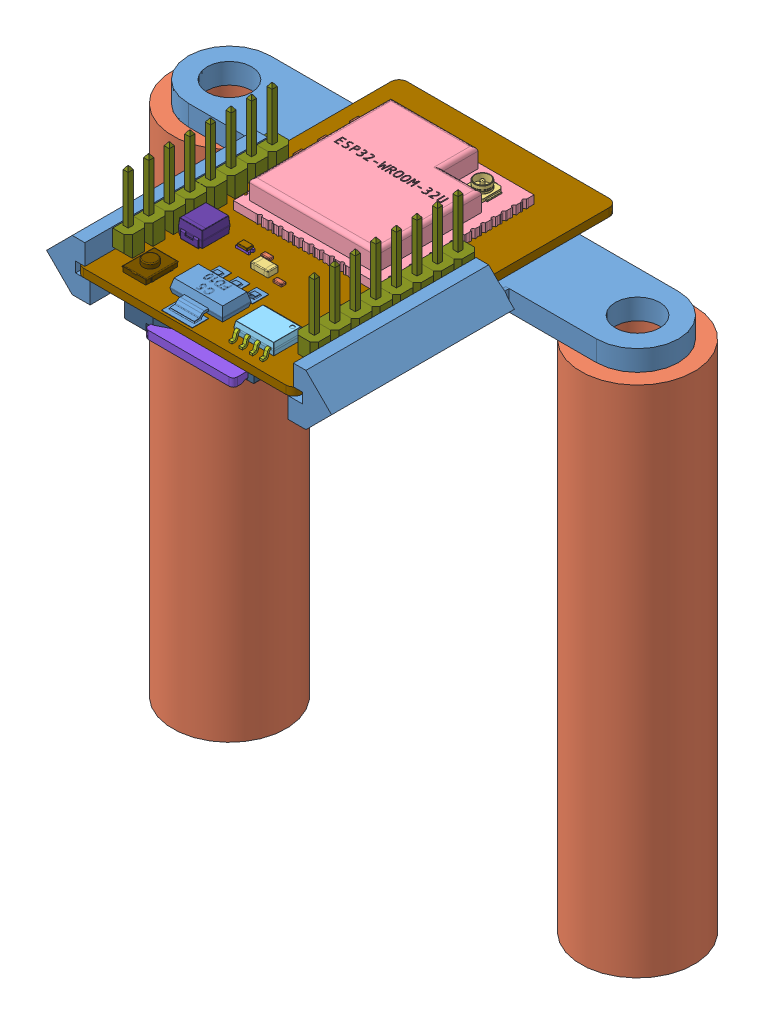
SolidWorks assembly camera_mount_fixed, configuration Default. Lengths in mm.
Overall size (64.5 76.05 40.5).
66 component instances, 27 part files, 7 mates.
Components (placement in the parent):
- camera_mount_mk1-1: camera_mount_mk1 [Default] at (-31.5868 36.0113 19.6726) x (-1 0 0) z (0 0 1) size (60.64 6.35 35.31)
- standoff_2.5-1: standoff_2.5 [Default] at (-19.7453 -31.2987 12.0526) size (14.02 63.5 14.02)
- standoff_2.5-2: standoff_2.5 [Default] at (-70.2252 -31.2987 12.0526) size (14.02 63.5 14.02)
- ESP3-CAM v5 - black pcb (1).step-1: ESP3-CAM v5 - black pcb (1).step [Default] at (-32.0188 35.7413 42.2786) x (0 0 -1) z (-1 0 0) size (40.5 18.08 27)
  - ESp32-WROOM-32U v3.step-1: ESp32-WROOM-32U v3.step [Default] at (15.3712 -0.1455 22.8712) x (0 0 -1) z (-1 0 0) size (18.07 3.43 19.24)
    - u.step-1: u.step [Default] at (15.6609 1 -15.1484) x (0 0 -1) z (1 0 0) size (3.1 1.25 3)
    - ESp32-WROOM-32U v3-0.step-1: ESp32-WROOM-32U v3-0.step [Default] at origin size (18.07 3.43 19.24)
  - sop127p-6mm-8 v2.step-1: sop127p-6mm-8 v2.step [Default] at (4 0 7) x (0 0 1) z (0 -1 0) size (4.9 5.9 1.65)
    - icbody.step-1: icbody.step [Default] at origin size (4.9 3.9 1.45)
    - Component5.step-1: Component5.step [Default] at origin size (0.4 1 1.05)
    - Component5.step-2: Component5.step [Default] at (1.27 0 0) size (0.4 1 1.05)
    - Component5.step-3: Component5.step [Default] at (-1.27 0 0) size (0.4 1 1.05)
    - Component5.step-4: Component5.step [Default] at (-2.54 0 0) size (0.4 1 1.05)
    - Component5(Mirror).step-1: Component5(Mirror).step [Default] at (-1.27 0 0) x (1 0 0) z (0 0 -1) size (0.4 1 1.05)
    - Component5(Mirror).step-2: Component5(Mirror).step [Default] at (1.27 0 0) x (1 0 0) z (0 0 -1) size (0.4 1 1.05)
    - Component5(Mirror).step-3: Component5(Mirror).step [Default] x (1 0 0) z (0 0 -1) size (0.4 1 1.05)
    - Component5(Mirror).step-4: Component5(Mirror).step [Default] at (-2.54 0 0) x (1 0 0) z (0 0 -1) size (0.4 1 1.05)
  - SMD LED 0603.step-1: SMD LED 0603.step [Default] at (12 0 18) x (0 0 1) z (0 -1 0) size (1.6 0.8 0.6)
    - Fusion.step-1: Fusion.step [Default] at origin size (1.6 0.8 0.5)
    - Fillet.step-1: Fillet.step [Default] at origin size (1.2 0.8 0.3)
  - MicroSD Slot.step-1: MicroSD Slot.step [Default] at (26.7 3 17.2) x (1 0 0) z (0 1 0) size (15 16 2)
    - sdreader.step-1: sdreader.step [Default] at (-11.2744 2.632 -3.2) size (15 16 2)
  - camera for ESP32.step-1: camera for ESP32.step [Default] at (24.1466 3.3198 13.5126) x (0 0 -1) z (0 1 0) size (12.5 21.5 6.03)
    - User Library-ov9655_ov9655_flex_pcb.step-1: User Library-ov9655_ov9655_flex_pcb.step [Default] at origin size (12.5 21.5 0.12)
    - User Library-ov9655_ov9655_flex_reinf.step-1: User Library-ov9655_ov9655_flex_reinf.step [Default] at origin size (12.5 4.5 0.25)
    - User Library-ov9655_ov9655_back_panel.step-1: User Library-ov9655_ov9655_back_panel.step [Default] at origin size (8.5 8.5 0.25)
    - User Library-ov9655_ov9655_body.step-1: User Library-ov9655_ov9655_body.step [Default] at origin size (8.5 8.5 6.03)
    - User Library-ov9655_ov9655_lens.step-1: User Library-ov9655_ov9655_lens.step [Default] at origin size (2 2 1.43)
  - Pin Header 4 x 1 TH 2.54mm Pitch.step-1: Pin Header 4 x 1 TH 2.54mm Pitch.step [Default] at (4.72 -2.6622 2.2022) x (0 0 1) z (0 1 0) size (2.54 10.16 11.43)
  - Pin Header 4 x 1 TH 2.54mm Pitch.step-2: Pin Header 4 x 1 TH 2.54mm Pitch.step [Default] at (14.883 -2.6622 2.2022) x (0 0 1) z (0 1 0) size (2.54 10.16 11.43)
  - Pin Header 4 x 1 TH 2.54mm Pitch.step-3: Pin Header 4 x 1 TH 2.54mm Pitch.step [Default] at (14.89 -2.6622 25.2022) x (0 0 1) z (0 1 0) size (2.54 10.16 11.43)
  - Pin Header 4 x 1 TH 2.54mm Pitch.step-4: Pin Header 4 x 1 TH 2.54mm Pitch.step [Default] at (4.71 -2.6622 25.2022) x (0 0 1) z (0 1 0) size (2.54 10.16 11.43)
  - capacitor-CAPM-TANTB-YL.step-1: capacitor-CAPM-TANTB-YL.step [Default] at (11 0.105 22.105) x (1 0 0) z (0 -1 0) size (3.7 3 2.1)
  - switch-3x4x2mm - 2 Pad.step-1: switch-3x4x2mm - 2 Pad.step [Default] at (4 0.685 21.7704) x (1 0 0) z (0 -1 0) size (5 3 1.93)
  - nano - reg.step-1: nano - reg.step [Default] at (4.45 -0.0047 14.7657) x (0 0 -1) z (-1 0 0) size (6.5 1.69 8.3)
  - resistor-NTC-0402-T0.6.step-1: resistor-NTC-0402-T0.6.step [Default] at (12.2 0 15.8) x (0 0 -1) z (1 0 0) size (1.1 0.55 0.6)
  - resistor-NTC-0402-T0.6.step-2: resistor-NTC-0402-T0.6.step [Default] at (10.2 0 12.3) x (0 0 -1) z (1 0 0) size (1.1 0.55 0.6)
  - resistor-NTC-0402-T0.6.step-3: resistor-NTC-0402-T0.6.step [Default] at (11.2 0 5.9714) x (0 0 -1) z (1 0 0) size (1.1 0.55 0.6)
  - resistor-NTC-0805-T1.3.step-1: resistor-NTC-0805-T1.3.step [Default] at (10.35 0 14.65) x (0 0 -1) z (1 0 0) size (2.2 1.4 1.3)
  - resistor-NTC-0402-T0.6.step-4: resistor-NTC-0402-T0.6.step [Default] at (4.5 0 10.6) x (-1 0 0) z (0 0 -1) size (1.1 0.55 0.6)
  - resistor-NTC-0402-T0.6.step-5: resistor-NTC-0402-T0.6.step [Default] at (25.5 0 24.5) size (1.1 0.55 0.6)
  - resistor-NTC-0402-T0.6.step-6: resistor-NTC-0402-T0.6.step [Default] at (28.5 0 24.5) size (1.1 0.55 0.6)
  - resistor-NTC-0402-T0.6.step-7: resistor-NTC-0402-T0.6.step [Default] at (32.5 0 24.5) size (1.1 0.55 0.6)
  - smd-transistor-SOT23-3.step-1: smd-transistor-SOT23-3.step [Default] at (27 1.058 2.442) x (1 0 0) z (0 1 0) size (2.84 3.01 1.19)
  - smd-transistor-SOT23-3.step-2: smd-transistor-SOT23-3.step [Default] at (27 1.058 23.942) x (1 0 0) z (0 1 0) size (2.84 3.01 1.19)
  - resistor-NTC-0402-T0.6.step-8: resistor-NTC-0402-T0.6.step [Default] at (29.3 1 24.3) x (0 0 1) z (-1 0 0) size (1.1 0.55 0.6)
  - resistor-NTC-0402-T0.6.step-9: resistor-NTC-0402-T0.6.step [Default] at (30.3 1 24.3) x (0 0 1) z (-1 0 0) size (1.1 0.55 0.6)
  - resistor-NTC-0402-T0.6.step-10: resistor-NTC-0402-T0.6.step [Default] at (31 1 17) size (1.1 0.55 0.6)
  - LED SMD 5050 White.step-1: LED SMD 5050 White.step [Default] at (30 1.2963 2.1003) x (1 0 0) z (0 1 0) size (5.4 5 1.62)
  - resistor-NTC-0402-T0.6.step-11: resistor-NTC-0402-T0.6.step [Default] at (20.7 1 4.3) x (0 0 -1) z (1 0 0) size (1.1 0.55 0.6)
  - resistor-NTC-0402-T0.6.step-12: resistor-NTC-0402-T0.6.step [Default] at (19.7 1 4.3) x (0 0 -1) z (1 0 0) size (1.1 0.55 0.6)
  - resistor-NTC-0402-T0.6.step-13: resistor-NTC-0402-T0.6.step [Default] at (18.7 1 4.3) x (0 0 -1) z (1 0 0) size (1.1 0.55 0.6)
  - resistor-NTC-0402-T0.6.step-14: resistor-NTC-0402-T0.6.step [Default] at (17.7 1 4.3) x (0 0 -1) z (1 0 0) size (1.1 0.55 0.6)
  - resistor-NTC-0402-T0.6.step-15: resistor-NTC-0402-T0.6.step [Default] at (21 1 5.2) size (1.1 0.55 0.6)
  - resistor-NTC-0402-T0.6.step-16: resistor-NTC-0402-T0.6.step [Default] at (18 1 6.2) size (1.1 0.55 0.6)
  - resistor-NTC-0402-T0.6.step-17: resistor-NTC-0402-T0.6.step [Default] at (18 1 7.2) size (1.1 0.55 0.6)
  - capacitor-CAPC-0603-T0.9-BN.step-1: capacitor-CAPC-0603-T0.9-BN.step [Default] at (21 1 7) size (1.7 0.9 0.9)
  - resistor-NTC-0402-T0.6.step-18: resistor-NTC-0402-T0.6.step [Default] at (21 1 6) size (1.1 0.55 0.6)
  - capacitor-CAPC-0603-T0.9-BN.step-2: capacitor-CAPC-0603-T0.9-BN.step [Default] at (22 1 21) size (1.7 0.9 0.9)
  - smd-transistor-SOT23-3.step-3: smd-transistor-SOT23-3.step [Default] at (21.5739 1.058 19.0158) x (0 0 -1) z (0 1 0) size (2.84 3.01 1.19)
  - connector smd usl00-20l_p0-4_l12-6_w2-75.step-1: connector smd usl00-20l_p0-4_l12-6_w2-75.step [Default] at (26.791 1 14.009) x (0 0 -1) z (1 0 0) size (12.6 1 3.1)
  - resistor-NTC-0402-T0.6.step-19: resistor-NTC-0402-T0.6.step [Default] at (18 1 14.2) size (1.1 0.55 0.6)
  - resistor-NTC-0402-T0.6.step-20: resistor-NTC-0402-T0.6.step [Default] at (18 1 13.2) size (1.1 0.55 0.6)
  - smd-transistor-SOT23-3.step-4: smd-transistor-SOT23-3.step [Default] at (21.5739 1.058 10.0158) x (0 0 -1) z (0 1 0) size (2.84 3.01 1.19)
  - Micro SD-Card.step-1: Micro SD-Card.step [Default] at (7 2.64 12.5) size (15 1.01 11)
  - ESP3-CAM.step-1: ESP3-CAM.step [Default] at origin size (40 1 27)
Mates (geometry in assembly coordinates):
- Coincident1: coincident anti-aligned: plane of camera_mount_mk1-1 through (-32.4123 32.2013 42.2786) normal (0 -1 0); plane of standoff_2.5-2 through (-67.0248 32.2013 12.0526) normal (0 1 0)
- Concentric1: concentric anti-aligned: circle of camera_mount_mk1-1; circle of standoff_2.5-2
- Concentric2: concentric anti-aligned: cylinder of camera_mount_mk1-1; cylinder of standoff_2.5-1 through (-19.7453 -31.2987 12.0526) axis (0 -1 0) radius 3.2004
- Coincident2: coincident anti-aligned: plane of camera_mount_mk1-1 through (-59.0188 34.7413 42.2786) normal (1 0 0); plane of ESP3-CAM v5 - black pcb (1).step-1/ESP3-CAM.step-1 through (-59.0188 35.7413 42.2786) normal (-1 0 0)
- Coincident3: coincident anti-aligned: plane of camera_mount_mk1-1 through (-31.5868 34.7413 42.2786) normal (0 1 0); plane of ESP3-CAM v5 - black pcb (1).step-1/ESP3-CAM.step-1 through (-45.5188 34.7413 22.2786) normal (0 -1 0)
- Parallel1: parallel anti-aligned: plane of camera_mount_mk1-1 through (-31.5868 36.0113 6.9726) normal (0 0 -1)
- Coincident4: coincident aligned: plane of camera_mount_mk1-1 through (-31.5868 36.0113 42.2786) normal (0 0 1); plane of ESP3-CAM v5 - black pcb (1).step-1/ESP3-CAM.step-1 through (-32.0188 35.7413 42.2786) normal (0 0 1)
